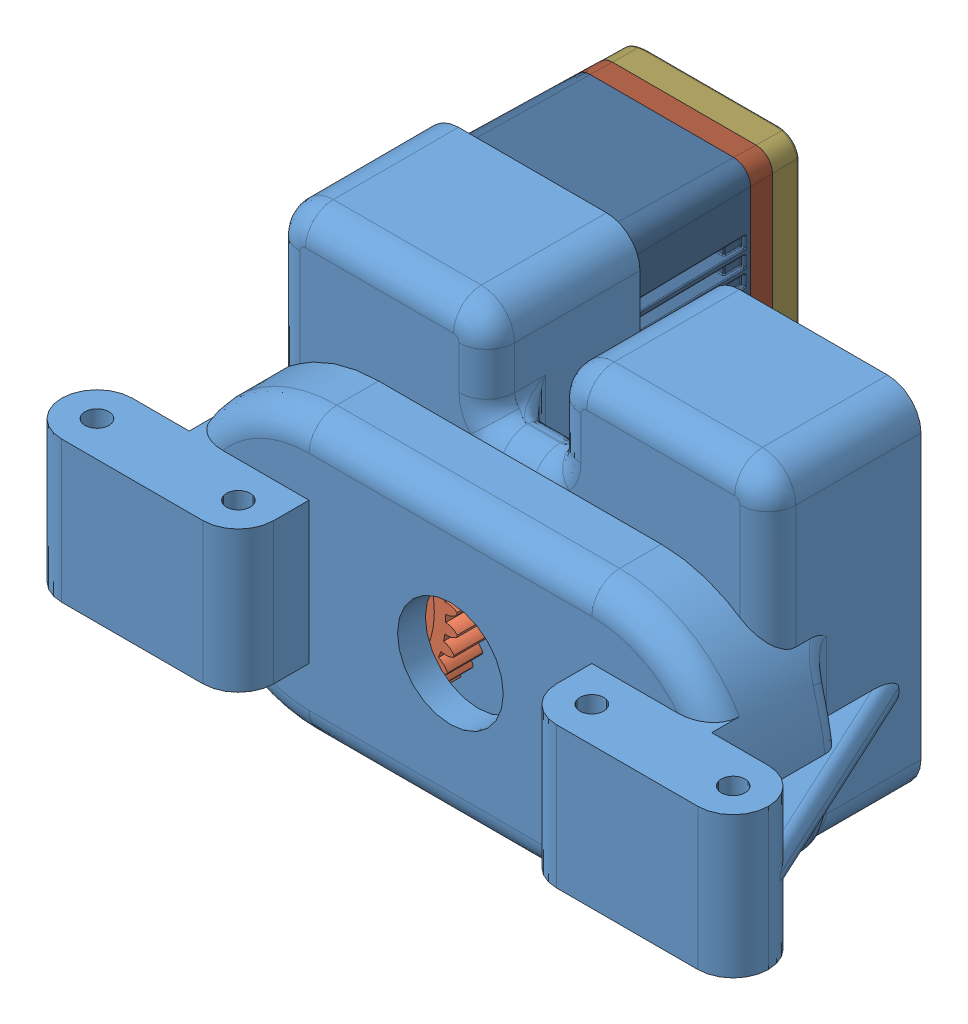
SolidWorks assembly Assem3, configuration Default. Lengths in mm.
Overall size (127 69.15 87.31).
24 component instances, 14 part files, 7 mates.
Components (placement in the parent):
- 2M_3to1_GearboxMark3-1: 2M_3to1_GearboxMark3 [Default] at (37.7483 57.6766 108.4215) size (127 69.15 52.7)
- 36T Gear (276-2169-002)-1: 36T Gear (276-2169-002) [Default] at (12.3483 57.6766 103.659) size (40.08 40.08 9.53)
- V5 Smart Motor (276-4840) no cap 3-1: V5 Smart Motor (276-4840) no cap 3 [Default] at (12.3483 70.3766 66.2215) x (0 -1 0) z (0 0 1) size (59.01 35.33 59.91)
  - V5 Smart Motor (276-4840).step-1: V5 Smart Motor (276-4840).step [Default] at origin size (59.01 35.33 59.91)
    - 276-4840-900 Rev6_Instruction.step-1: 276-4840-900 Rev6_Instruction.step [Default] at (-14.3 0 -17.2) size (52.79 15.94 38.15)
      - 276-4840-901 Rev6.step-1: 276-4840-901 Rev6.step [Default] at (10.75 -10.05 17.8) x (-1 0 0) z (0 0 1) size (49.9 1.6 38.15)
      - 276-4840-902 Rev2.step-1: 276-4840-902 Rev2.step [Default] at (31.25 -9.25 6.2) x (0 0 -1) z (0 -1 0) size (10.35 11.39 15.94)
      - 276-4840-022 Rev4.step-1: 276-4840-022 Rev4.step [Default] at (31.25 -9.25 6.2) x (0 0 -1) z (1 0 0) size (10.26 9.1 5.51)
    - 276-4840-110 Rev10_Instruction.step-1: 276-4840-110 Rev10_Instruction.step [Default] at (12.7 0 14.7) size (35.33 35.33 31.1)
      - 276-4840-061 Rev7_Ring_Gear_Fixed01 .6 Rev3.step-1: 276-4840-061 Rev7_Ring_Gear_Fixed01 .6 Rev3.step [Default] at origin size (28.79 28.39 24.6)
      - 276-4840-018 Rev6.step-1: 276-4840-018 Rev6.step [Default] at (0 0 6.7) x (-0.483174 0.875524 0) z (0 0 1) size (26 26 12.3)
      - 276-4840-059 Rev2.step-1: 276-4840-059 Rev2.step [Default] at (0 0 10.3) size (28.4 28.4 8.5)
      - 276-4840-062 Rev1.step-1: 276-4840-062 Rev1.step [Default] at (-12.1353 8.8168 12.3) x (0.956835 -0.290632 0) z (-0.290632 -0.956835 0) size (3.2 6.56 3.2)
      - 276-4840-062 Rev1.step-2: 276-4840-062 Rev1.step [Default] at (12.1353 8.8168 12.3) x (0.978427 0.206591 0) z (0.206591 -0.978427 0) size (3.2 6.56 3.2)
      - 276-4840-062 Rev1.step-3: 276-4840-062 Rev1.step [Default] at (-12.1353 -8.8168 12.3) x (0.72563 0.688086 0) z (0.688086 -0.72563 0) size (3.2 6.56 3.2)
    - 276-4840-001 Rev38.step-1: 276-4840-001 Rev38.step [Default] at origin size (57.3 33 46.9)
    - 276-4840-005 Rev27.step-1: 276-4840-005 Rev27.step [Default] at (0 0 -17.95) size (56.17 31.87 12.9)
    - 276-4840-004 Rev16.step-1: 276-4840-004 Rev16.step [Default] at (0 0 -19.2) size (56.01 31.71 9.21)
    - 276-4840-009 Rev3.step-1: 276-4840-009 Rev3.step [Default] at (25.45 13.5 15.7) x (0.19987 -0.979823 0) z (-0.979823 -0.19987 0) size (3.4 41.31 4.34)
    - 276-4840-009 Rev3.step-2: 276-4840-009 Rev3.step [Default] at (-25.45 -13.5 15.7) x (-0.998855 0.047836 0) z (0.047836 0.998855 0) size (3.4 41.31 4.34)
    - 276-4840-009 Rev3.step-3: 276-4840-009 Rev3.step [Default] at (25.45 -13.5 15.7) x (-0.975374 0.220559 0) z (0.220559 0.975374 0) size (3.4 41.31 4.34)
    - 276-4840-009 Rev3.step-4: 276-4840-009 Rev3.step [Default] at (-25.45 13.5 15.7) x (-0.922256 0.38658 0) z (0.38658 0.922256 0) size (3.4 41.31 4.34)
    - 276-4840-025 Rev19.step-1: 276-4840-025 Rev19.step [Default] at (12.7 0 -22.63) x (-0.993315 0.115437 0) z (0 0 1) size (14.82 14.83 35.18)
- 36T Gear (276-2169-002)-2: 36T Gear (276-2169-002) [Default] at (62.6778 57.9336 103.659) size (40.08 40.08 9.53)
Mates (geometry in assembly coordinates):
- Concentric1: concentric anti-aligned: circle of 36T Gear (276-2169-002)-1; circle of 2M_3to1_GearboxMark3-1
- Coincident1: coincident anti-aligned: plane of 2M_3to1_GearboxMark3-1 through (37.7483 57.6766 108.4215) normal (0 0 -1); plane of 36T Gear (276-2169-002)-1 through (12.3483 57.6766 108.4215) normal (0 0 1)
- Concentric2: concentric aligned: circle of 2M_3to1_GearboxMark3-1; circle of V5 Smart Motor (276-4840) no cap 3-1/V5 Smart Motor (276-4840).step-1/276-4840-110 Rev10_Instruction.step-1/276-4840-059 Rev2.step-1
- Parallel1: parallel anti-aligned: line of 2M_3to1_GearboxMark3-1 through (-0.8017 99.4266 83.4215) axis (1 0 0); line of V5 Smart Motor (276-4840) no cap 3-1/V5 Smart Motor (276-4840).step-1/276-4840-001 Rev38.step-1 through (25.2483 99.0266 82.4215) axis (-1 0 0)
- Parallel2: parallel anti-aligned: line of 2M_3to1_GearboxMark3-1 through (-4.4017 45.0266 83.4215) axis (0 1 0); line of V5 Smart Motor (276-4840) no cap 3-1/V5 Smart Motor (276-4840).step-1/276-4840-001 Rev38.step-1 through (-3.1692 92.5266 83.4215) axis (0 -1 0)
- Coincident6: coincident anti-aligned: plane of 2M_3to1_GearboxMark3-1 through (37.7483 57.6766 83.4215) normal (0 0 -1); plane of V5 Smart Motor (276-4840) no cap 3-1/V5 Smart Motor (276-4840).step-1/276-4840-001 Rev38.step-1 through (25.2483 95.4266 83.4215) normal (0 0 1)
- Coincident7: coincident anti-aligned: plane of 2M_3to1_GearboxMark3-1 through (37.7483 57.6766 108.4215) normal (0 0 -1); plane of 36T Gear (276-2169-002)-2 through (62.6778 57.9336 108.4215) normal (0 0 1)
